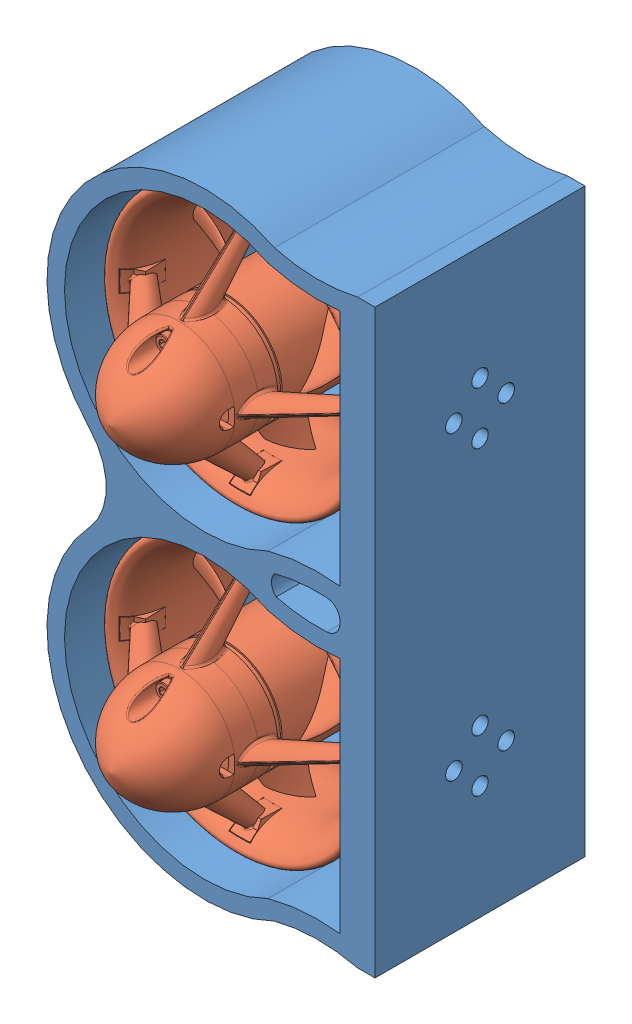
SolidWorks assembly CR-A-0004b-VerticalMotorAssem, configuration Default. Lengths in mm.
Overall size (119.06 223.52 112.68).
3 component instances, 2 part files, 6 mates.
Components (placement in the parent):
- CR-P-0005b-Frame-MotorMount Vertical-1: CR-P-0005b-Frame-MotorMount Vertical [Default] at (65.652 113.9901 182.7577) size (119.06 223.52 78.04)
- CR-P-0003-T200-THRUSTER-R1-1: CR-P-0003-T200-THRUSTER-R1 [Default] at (65.8645 223.2101 226.1095) x (0 -1 0) z (0 0 1) size (96.71 97.53 112.68)
- CR-P-0003-T200-THRUSTER-R1-2: CR-P-0003-T200-THRUSTER-R1 [Default] at (65.8645 113.9901 226.1095) x (0 -1 0) z (0 0 1) size (96.71 97.53 112.68)
Mates (geometry in assembly coordinates):
- Coincident2: coincident anti-aligned: plane of CR-P-0005b-Frame-MotorMount Vertical-1 through (114.8645 113.9901 258.9577) normal (-1 0 0); plane of CR-P-0003-T200-THRUSTER-R1-2 through (114.8645 113.9901 220.8577) normal (1 0 0)
- Coincident6: coincident anti-aligned: plane of CR-P-0005b-Frame-MotorMount Vertical-1 through (114.8645 113.9901 258.9577) normal (-1 0 0); plane of CR-P-0003-T200-THRUSTER-R1-1 through (114.8645 223.2101 220.8577) normal (1 0 0)
- Concentric9: concentric anti-aligned: circle of CR-P-0005b-Frame-MotorMount Vertical-1; circle of CR-P-0003-T200-THRUSTER-R1-2
- Concentric13: concentric anti-aligned: circle of CR-P-0005b-Frame-MotorMount Vertical-1; circle of CR-P-0003-T200-THRUSTER-R1-2
- Concentric14: concentric aligned: circle of CR-P-0005b-Frame-MotorMount Vertical-1; circle of CR-P-0003-T200-THRUSTER-R1-1
- Concentric15: concentric aligned: circle of CR-P-0005b-Frame-MotorMount Vertical-1; circle of CR-P-0003-T200-THRUSTER-R1-1
